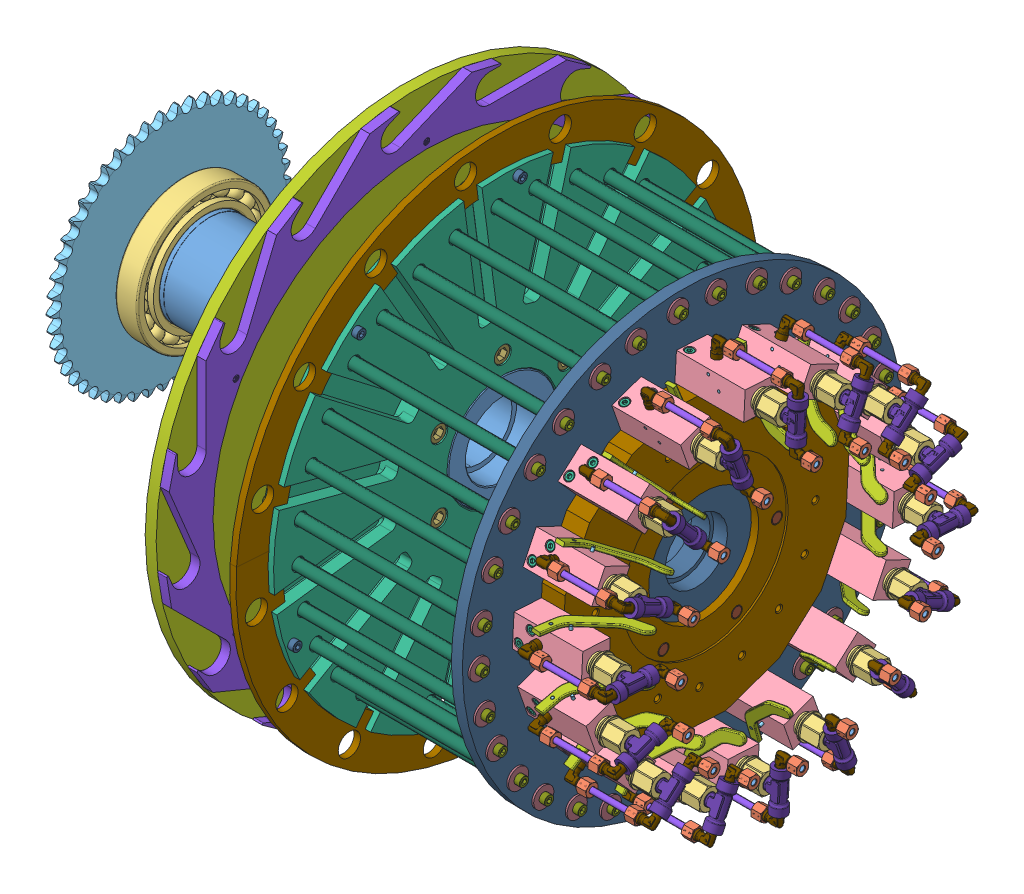
SolidWorks assembly assieme parte rotante, configuration Default. Lengths in mm.
Overall size (749.63 778.63 778.63).
555 component instances, 28 part files, 76 mates.
Components (placement in the parent):
- albero rotazione piatti-1: albero rotazione piatti [Default] at (60.413 18.3637 415) size (415 200 200)
- c-type retaining ring_external_ks-1: c-type retaining ring_external_ks [KS 1336 E - 100] at (-146.4567 18.3637 415) x (0 0 -1) z (1 0 0) size (107.55 112.98 3)
- SKF - 6020 - 20,DE,NC,20_68-1: SKF - 6020 - 20,DE,NC,20_68 [SKF - 6020 - 20,DE,NC,20_68] at (-131.4567 18.3637 415) x (1 0 0) z (0 -0.434476 -0.900684) size (24 150 150)
- calettatore d95-1: calettatore d95 [Default] at (-173.8867 18.3637 415) size (39.5 135 135)
- Chain wheel ISO - 50Z 10A-1-1: Chain wheel ISO - 50Z 10A-1 [Chain wheel ISO - 50Z 10A-1 --50SB120H25L95.0N] at (-164.8867 18.3637 415) size (29.89 262.06 262.51)
- Disco supporto montaggio e Colonne-1: Disco supporto montaggio e Colonne [Default] at (204.0433 18.3637 415) x (0 -0.866025 -0.5) z (1 0 0) size (499.6 499.6 29)
- SKF - 6020 - 20,DE,NC,20_68-2: SKF - 6020 - 20,DE,NC,20_68 [SKF - 6020 - 20,DE,NC,20_68] at (62.0433 18.3637 415) x (1 0 0) z (0 -0.432628 -0.901573) size (24 150 150)
- piatto rotante porta tappi-1: piatto rotante porta tappi [Default] at (99.0433 18.3637 415) x (0 0 -1) z (1 0 0) size (570 570 20.57)
- disco trasportatore tappi 31-1: disco trasportatore tappi 31 [Default] at (111.0433 18.3637 415) x (0 0.5 -0.866025) z (1 0 0) size (570 570 10.42)
- Distributore Rotante-1: Distributore Rotante [Default] at (425.0433 18.3637 415) x (0 -0.055301 -0.99847) z (1 0 0) size (310 310 25.54)
- disco trascinato porta distributore vuoto-1: disco trascinato porta distributore vuoto [Default] at (400.0433 18.3637 415) x (0 0.055301 0.99847) z (-1 0 0) size (480 480 50)
- m12 35mm-1: m12 35mm [ISO 4762 M12 x 35 - 35N] at (376.0433 -53.0243 378.8925) x (1 0 0) z (0 -0.5 0.866025) size (47 18 18)
- m12 90mm-3: m12 90mm [ISO 4762 M12 x 90 - 90N] at (203.0433 -21.6363 345.718) x (-1 0 0) z (0 -0.5 0.866025) size (102 18 18)
- plain washer xlarge grade c_iso-1: plain washer xlarge grade c_iso [Washer ISO 7094 - 6] at (99.0433 -101.6363 207.1539) x (1 0 0) z (0 -1 0) size (2 22 22)
- M6 20mm-1: M6 20mm [ISO 4762 M6 x 20 - 20N] at (91.0433 -101.6363 207.1539) x (1 0 0) z (0 0.5 0.866025) size (26 10 10)
- m12 35mm-2: m12 35mm [ISO 4762 M12 x 35 - 35N] at (376.0433 13.9397 335.1224) x (1 0 0) z (0 -1 0) size (47 18 18)
- m12 35mm-3: m12 35mm [ISO 4762 M12 x 35 - 35N] at (376.0433 85.3277 371.2299) x (1 0 0) z (0 -0.5 -0.866025) size (47 18 18)
- m12 35mm-4: m12 35mm [ISO 4762 M12 x 35 - 35N] at (376.0433 89.7517 451.1075) x (1 0 0) z (0 0.5 -0.866025) size (47 18 18)
- m12 35mm-5: m12 35mm [ISO 4762 M12 x 35 - 35N] at (376.0433 22.7877 494.8776) x (1 0 0) z (0 1 0) size (47 18 18)
- m12 35mm-6: m12 35mm [ISO 4762 M12 x 35 - 35N] at (376.0433 -48.6003 458.7701) x (1 0 0) z (0 0.5 0.866025) size (47 18 18)
- plain washer xlarge grade c_iso-2: plain washer xlarge grade c_iso [Washer ISO 7094 - 6] at (99.0433 138.3637 207.1539) x (1 0 0) z (0 -0.5 -0.866025) size (2 22 22)
- plain washer xlarge grade c_iso-3: plain washer xlarge grade c_iso [Washer ISO 7094 - 6] at (99.0433 258.3637 415) x (1 0 0) z (0 0.5 -0.866025) size (2 22 22)
- plain washer xlarge grade c_iso-4: plain washer xlarge grade c_iso [Washer ISO 7094 - 6] at (99.0433 138.3637 622.8461) x (1 0 0) z (0 1 0) size (2 22 22)
- plain washer xlarge grade c_iso-5: plain washer xlarge grade c_iso [Washer ISO 7094 - 6] at (99.0433 -101.6363 622.8461) x (1 0 0) z (0 0.5 0.866025) size (2 22 22)
- plain washer xlarge grade c_iso-6: plain washer xlarge grade c_iso [Washer ISO 7094 - 6] at (99.0433 -221.6363 415) x (1 0 0) z (0 -0.5 0.866025) size (2 22 22)
- M6 20mm-2: M6 20mm [ISO 4762 M6 x 20 - 20N] at (91.0433 138.3637 207.1539) x (1 0 0) z (0 -0.5 0.866025) size (26 10 10)
- M6 20mm-3: M6 20mm [ISO 4762 M6 x 20 - 20N] at (91.0433 258.3637 415) x (1 0 0) z (0 -1 0) size (26 10 10)
- M6 20mm-4: M6 20mm [ISO 4762 M6 x 20 - 20N] at (91.0433 138.3637 622.8461) x (1 0 0) z (0 -0.5 -0.866025) size (26 10 10)
- M6 20mm-5: M6 20mm [ISO 4762 M6 x 20 - 20N] at (91.0433 -101.6363 622.8461) x (1 0 0) z (0 0.5 -0.866025) size (26 10 10)
- M6 20mm-6: M6 20mm [ISO 4762 M6 x 20 - 20N] at (91.0433 -221.6363 415) x (1 0 0) z (0 1 0) size (26 10 10)
- m12 90mm-4: m12 90mm [ISO 4762 M12 x 90 - 90N] at (203.0433 58.3637 345.718) x (-1 0 0) z (0 -1 0) size (102 18 18)
- m12 90mm-5: m12 90mm [ISO 4762 M12 x 90 - 90N] at (203.0433 98.3637 415) x (-1 0 0) z (0 -0.5 -0.866025) size (102 18 18)
- m12 90mm-6: m12 90mm [ISO 4762 M12 x 90 - 90N] at (203.0433 58.3637 484.282) x (-1 0 0) z (0 0.5 -0.866025) size (102 18 18)
- m12 90mm-7: m12 90mm [ISO 4762 M12 x 90 - 90N] at (203.0433 -21.6363 484.282) x (-1 0 0) z (0 1 0) size (102 18 18)
- m12 90mm-8: m12 90mm [ISO 4762 M12 x 90 - 90N] at (203.0433 -61.6363 415) x (-1 0 0) z (0 0.5 0.866025) size (102 18 18)
- asta scorrimento carello-1: asta scorrimento carello [Default] at (287.5433 70.1437 197.9013) x (0 0 -1) z (1 0 0) size (12 12 225)
- plain washer xlarge grade c_iso-7: plain washer xlarge grade c_iso [Washer ISO 7094 - 6] at (175.0433 70.1437 197.9013) x (1 0 0) z (0 -1 0) size (2 22 22)
- M6 16mm-1: M6 16mm [ISO 4762 M6 x 16 - 16N] at (167.0433 70.1437 197.9013) size (22 10 10)
- M6 16mm-2: M6 16mm [ISO 4762 M6 x 16 - 16N] at (408.0433 70.1437 197.9013) x (-1 0 0) z (0 0 -1) size (22 10 10)
- plain washer xlarge grade c_iso-26: plain washer xlarge grade c_iso [Washer ISO 7094 - 6] at (400.0433 70.1437 197.9013) x (-1 0 0) z (0 1 0) size (2 22 22)
- plain washer xlarge grade c_iso-42: plain washer xlarge grade c_iso [Washer ISO 7094 - 6] at (175.0433 24.5373 191.8971) x (1 0 0) z (0 -0.965926 -0.258819) size (2 22 22)
- M6 16mm-3: M6 16mm [ISO 4762 M6 x 16 - 16N] at (167.0433 24.5373 191.8971) x (1 0 0) z (0 0.258819 -0.965926) size (22 10 10)
- asta scorrimento carello-2: asta scorrimento carello [Default] at (287.5433 24.5373 191.8971) x (0 0.258819 -0.965926) z (-1 0 0) size (12 12 225)
- plain washer xlarge grade c_iso-58: plain washer xlarge grade c_iso [Washer ISO 7094 - 6] at (400.0433 24.5373 191.8971) x (-1 0 0) z (0 0.965926 0.258819) size (2 22 22)
- M6 16mm-4: M6 16mm [ISO 4762 M6 x 16 - 16N] at (408.0433 24.5373 191.8971) x (-1 0 0) z (0 -0.258819 0.965926) size (22 10 10)
- AssiemeValvola-1: AssiemeValvola [Default] at (515.3257 74.6348 254.5832) x (0 -0.331007 0.943628) z (0 0.943628 0.331007) size (90.26 138.63 38)
  - RaccordoT-1: RaccordoT [Default] at origin size (43 29.75 16.5)
  - Raccordo a L-1: Raccordo a L [Default] at (-30 0 0) x (0 -1 0) z (0 0 -1) size (28.34 25.51 14.01)
    - 1809_06_10_01-1: 1809_06_10_01 [Default] at origin size (22.49 23 10)
    - 1809_06_10_02-1: 1809_06_10_02 [Default] at origin size (6.5 8.5 8.5)
    - 1809_06_10_03-1: 1809_06_10_03 [Default] at origin size (11.02 15.01 14.01)
  - Raccordo a L-2: Raccordo a L [Default] at (30 0 0) x (0 1 0) z (0 0 -1) size (28.34 25.51 14.01)
    - 1809_06_10_01-1: 1809_06_10_01 [Default] at origin size (22.49 23 10)
    - 1809_06_10_02-1: 1809_06_10_02 [Default] at origin size (6.5 8.5 8.5)
    - 1809_06_10_03-1: 1809_06_10_03 [Default] at origin size (11.02 15.01 14.01)
  - TappoChiusura-1: TappoChiusura [Default] at (0 -32 0) x (0 -1 0) z (0 0 1) size (38.28 26.74 26.74)
  - CorpoValvola-1: CorpoValvola [Default] at (-15 -115.2824 0) size (30 75 34)
  - Raccordo a L-3: Raccordo a L [Default] at (-30 -88.2824 0) x (0 1 0) z (0 0 1) size (28.34 25.51 14.01)
    - 1809_06_10_01-1: 1809_06_10_01 [Default] at origin size (22.49 23 10)
    - 1809_06_10_02-1: 1809_06_10_02 [Default] at origin size (6.5 8.5 8.5)
    - 1809_06_10_03-1: 1809_06_10_03 [Default] at origin size (11.02 15.01 14.01)
  - Spina_3x38-1: Spina_3x38 [Default] at (0 -68.2824 -21) x (-1 0 0) z (0 0 1) size (3 3 38)
  - Spina_3x38-2: Spina_3x38 [Default] at (-10 -80.2824 -21) x (0.996193 0.087174 0) z (0 0 1) size (3 3 38)
  - M5 40mm-3: M5 40mm [ISO 4762 M5 x 40 - 40N] at (-14.6 -108.7824 9) size (45 8.5 8.5)
  - M5 40mm-2: M5 40mm [ISO 4762 M5 x 40 - 40N] at (-14.6 -96.7824 -9) size (45 8.5 8.5)
  - LevaValvola-1: LevaValvola [Default] at (-24.507 -86.571 -17) x (0.996193 0.087174 0) z (0 0 1) size (77.55 60.2 4)
  - Tubo-1: Tubo [Default] at (-30 -15.9665 0) x (1 0 0) z (0 -1 0) size (6 6 56.4)
- M6 16mm-5: M6 16mm [ISO 4762 M6 x 16 - 16N] at (167.0433 -16.8778 194.6116) x (1 0 0) z (0 0.382683 0.92388) size (22 10 10)
- M6 16mm-6: M6 16mm [ISO 4762 M6 x 16 - 16N] at (167.0433 -98.5342 224.874) x (1 0 0) z (0 0.707107 0.707107) size (22 10 10)
- M6 16mm-7: M6 16mm [ISO 4762 M6 x 16 - 16N] at (167.0433 -162.3939 284.0814) x (1 0 0) z (0 0.92388 0.382683) size (22 10 10)
- M6 16mm-8: M6 16mm [ISO 4762 M6 x 16 - 16N] at (167.0433 -198.735 363.22) x (1 0 0) z (0 1 0) size (22 10 10)
- M6 16mm-9: M6 16mm [ISO 4762 M6 x 16 - 16N] at (167.0433 -202.0247 450.2415) x (1 0 0) z (0 0.92388 -0.382683) size (22 10 10)
- M6 16mm-10: M6 16mm [ISO 4762 M6 x 16 - 16N] at (167.0433 -171.7623 531.8979) x (1 0 0) z (0 0.707107 -0.707107) size (22 10 10)
- M6 16mm-11: M6 16mm [ISO 4762 M6 x 16 - 16N] at (167.0433 -112.5549 595.7576) x (1 0 0) z (0 0.382683 -0.92388) size (22 10 10)
- M6 16mm-12: M6 16mm [ISO 4762 M6 x 16 - 16N] at (167.0433 -33.4163 632.0987) x (1 0 0) z (0 0 -1) size (22 10 10)
- M6 16mm-13: M6 16mm [ISO 4762 M6 x 16 - 16N] at (167.0433 53.6052 635.3884) x (1 0 0) z (0 -0.382683 -0.92388) size (22 10 10)
- M6 16mm-14: M6 16mm [ISO 4762 M6 x 16 - 16N] at (167.0433 135.2616 605.126) x (1 0 0) z (0 -0.707107 -0.707107) size (22 10 10)
- M6 16mm-15: M6 16mm [ISO 4762 M6 x 16 - 16N] at (167.0433 199.1213 545.9186) x (1 0 0) z (0 -0.92388 -0.382683) size (22 10 10)
- M6 16mm-16: M6 16mm [ISO 4762 M6 x 16 - 16N] at (167.0433 235.4624 466.78) x (1 0 0) z (0 -1 0) size (22 10 10)
- M6 16mm-17: M6 16mm [ISO 4762 M6 x 16 - 16N] at (167.0433 238.7521 379.7585) x (1 0 0) z (0 -0.92388 0.382683) size (22 10 10)
- M6 16mm-18: M6 16mm [ISO 4762 M6 x 16 - 16N] at (167.0433 208.4897 298.1021) x (1 0 0) z (0 -0.707107 0.707107) size (22 10 10)
- M6 16mm-19: M6 16mm [ISO 4762 M6 x 16 - 16N] at (167.0433 149.2823 234.2424) x (1 0 0) z (0 -0.382683 0.92388) size (22 10 10)
- plain washer xlarge grade c_iso-11: plain washer xlarge grade c_iso [Washer ISO 7094 - 6] at (175.0433 -16.8778 194.6116) x (1 0 0) z (0 -0.92388 0.382683) size (2 22 22)
- plain washer xlarge grade c_iso-12: plain washer xlarge grade c_iso [Washer ISO 7094 - 6] at (175.0433 -98.5342 224.874) x (1 0 0) z (0 -0.707107 0.707107) size (2 22 22)
- plain washer xlarge grade c_iso-13: plain washer xlarge grade c_iso [Washer ISO 7094 - 6] at (175.0433 -162.3939 284.0814) x (1 0 0) z (0 -0.382683 0.92388) size (2 22 22)
- plain washer xlarge grade c_iso-14: plain washer xlarge grade c_iso [Washer ISO 7094 - 6] at (175.0433 -198.735 363.22) size (2 22 22)
- plain washer xlarge grade c_iso-15: plain washer xlarge grade c_iso [Washer ISO 7094 - 6] at (175.0433 -202.0247 450.2415) x (1 0 0) z (0 0.382683 0.92388) size (2 22 22)
- plain washer xlarge grade c_iso-16: plain washer xlarge grade c_iso [Washer ISO 7094 - 6] at (175.0433 -171.7623 531.8979) x (1 0 0) z (0 0.707107 0.707107) size (2 22 22)
- plain washer xlarge grade c_iso-17: plain washer xlarge grade c_iso [Washer ISO 7094 - 6] at (175.0433 -112.5549 595.7576) x (1 0 0) z (0 0.92388 0.382683) size (2 22 22)
- plain washer xlarge grade c_iso-18: plain washer xlarge grade c_iso [Washer ISO 7094 - 6] at (175.0433 -33.4163 632.0987) x (1 0 0) z (0 1 0) size (2 22 22)
- plain washer xlarge grade c_iso-19: plain washer xlarge grade c_iso [Washer ISO 7094 - 6] at (175.0433 53.6052 635.3884) x (1 0 0) z (0 0.92388 -0.382683) size (2 22 22)
- plain washer xlarge grade c_iso-20: plain washer xlarge grade c_iso [Washer ISO 7094 - 6] at (175.0433 135.2616 605.126) x (1 0 0) z (0 0.707107 -0.707107) size (2 22 22)
- plain washer xlarge grade c_iso-21: plain washer xlarge grade c_iso [Washer ISO 7094 - 6] at (175.0433 199.1213 545.9186) x (1 0 0) z (0 0.382683 -0.92388) size (2 22 22)
- plain washer xlarge grade c_iso-22: plain washer xlarge grade c_iso [Washer ISO 7094 - 6] at (175.0433 235.4624 466.78) x (1 0 0) z (0 0 -1) size (2 22 22)
- plain washer xlarge grade c_iso-23: plain washer xlarge grade c_iso [Washer ISO 7094 - 6] at (175.0433 238.7521 379.7585) x (1 0 0) z (0 -0.382683 -0.92388) size (2 22 22)
- plain washer xlarge grade c_iso-24: plain washer xlarge grade c_iso [Washer ISO 7094 - 6] at (175.0433 208.4897 298.1021) x (1 0 0) z (0 -0.707107 -0.707107) size (2 22 22)
- plain washer xlarge grade c_iso-25: plain washer xlarge grade c_iso [Washer ISO 7094 - 6] at (175.0433 149.2823 234.2424) x (1 0 0) z (0 -0.92388 -0.382683) size (2 22 22)
- asta scorrimento carello-3: asta scorrimento carello [Default] at (287.5433 -16.8778 194.6116) x (0 -0.382683 -0.92388) z (1 0 0) size (12 12 225)
- asta scorrimento carello-4: asta scorrimento carello [Default] at (287.5433 -98.5342 224.874) x (0 -0.707107 -0.707107) z (1 0 0) size (12 12 225)
- asta scorrimento carello-5: asta scorrimento carello [Default] at (287.5433 -162.3939 284.0814) x (0 -0.92388 -0.382683) z (1 0 0) size (12 12 225)
- asta scorrimento carello-6: asta scorrimento carello [Default] at (287.5433 -198.735 363.22) x (0 -1 0) z (1 0 0) size (12 12 225)
- asta scorrimento carello-7: asta scorrimento carello [Default] at (287.5433 -202.0247 450.2415) x (0 -0.92388 0.382683) z (1 0 0) size (12 12 225)
- asta scorrimento carello-8: asta scorrimento carello [Default] at (287.5433 -171.7623 531.8979) x (0 -0.707107 0.707107) z (1 0 0) size (12 12 225)
- asta scorrimento carello-9: asta scorrimento carello [Default] at (287.5433 -112.5549 595.7576) x (0 -0.382683 0.92388) z (1 0 0) size (12 12 225)
- asta scorrimento carello-10: asta scorrimento carello [Default] at (287.5433 -33.4163 632.0987) x (0 0 1) z (1 0 0) size (12 12 225)
- asta scorrimento carello-11: asta scorrimento carello [Default] at (287.5433 53.6052 635.3884) x (0 0.382683 0.92388) z (1 0 0) size (12 12 225)
- asta scorrimento carello-12: asta scorrimento carello [Default] at (287.5433 135.2616 605.126) x (0 0.707107 0.707107) z (1 0 0) size (12 12 225)
- asta scorrimento carello-13: asta scorrimento carello [Default] at (287.5433 199.1213 545.9186) x (0 0.92388 0.382683) z (1 0 0) size (12 12 225)
- asta scorrimento carello-14: asta scorrimento carello [Default] at (287.5433 235.4624 466.78) x (0 1 0) z (1 0 0) size (12 12 225)
- asta scorrimento carello-15: asta scorrimento carello [Default] at (287.5433 238.7521 379.7585) x (0 0.92388 -0.382683) z (1 0 0) size (12 12 225)
- asta scorrimento carello-16: asta scorrimento carello [Default] at (287.5433 208.4897 298.1021) x (0 0.707107 -0.707107) z (1 0 0) size (12 12 225)
- asta scorrimento carello-17: asta scorrimento carello [Default] at (287.5433 149.2823 234.2424) x (0 0.382683 -0.92388) z (1 0 0) size (12 12 225)
- M6 16mm-20: M6 16mm [ISO 4762 M6 x 16 - 16N] at (408.0433 -16.8778 194.6116) x (-1 0 0) z (0 -0.382683 -0.92388) size (22 10 10)
- M6 16mm-21: M6 16mm [ISO 4762 M6 x 16 - 16N] at (408.0433 -98.5342 224.874) x (-1 0 0) z (0 -0.707107 -0.707107) size (22 10 10)
- M6 16mm-22: M6 16mm [ISO 4762 M6 x 16 - 16N] at (408.0433 -162.3939 284.0814) x (-1 0 0) z (0 -0.92388 -0.382683) size (22 10 10)
- M6 16mm-23: M6 16mm [ISO 4762 M6 x 16 - 16N] at (408.0433 -198.735 363.22) x (-1 0 0) z (0 -1 0) size (22 10 10)
- M6 16mm-24: M6 16mm [ISO 4762 M6 x 16 - 16N] at (408.0433 -202.0247 450.2415) x (-1 0 0) z (0 -0.92388 0.382683) size (22 10 10)
- M6 16mm-25: M6 16mm [ISO 4762 M6 x 16 - 16N] at (408.0433 -171.7623 531.8979) x (-1 0 0) z (0 -0.707107 0.707107) size (22 10 10)
- M6 16mm-26: M6 16mm [ISO 4762 M6 x 16 - 16N] at (408.0433 -112.5549 595.7576) x (-1 0 0) z (0 -0.382683 0.92388) size (22 10 10)
- M6 16mm-27: M6 16mm [ISO 4762 M6 x 16 - 16N] at (408.0433 -33.4163 632.0987) x (-1 0 0) z (0 0 1) size (22 10 10)
- M6 16mm-28: M6 16mm [ISO 4762 M6 x 16 - 16N] at (408.0433 53.6052 635.3884) x (-1 0 0) z (0 0.382683 0.92388) size (22 10 10)
- M6 16mm-29: M6 16mm [ISO 4762 M6 x 16 - 16N] at (408.0433 135.2616 605.126) x (-1 0 0) z (0 0.707107 0.707107) size (22 10 10)
- M6 16mm-30: M6 16mm [ISO 4762 M6 x 16 - 16N] at (408.0433 199.1213 545.9186) x (-1 0 0) z (0 0.92388 0.382683) size (22 10 10)
- M6 16mm-31: M6 16mm [ISO 4762 M6 x 16 - 16N] at (408.0433 235.4624 466.78) x (-1 0 0) z (0 1 0) size (22 10 10)
- M6 16mm-32: M6 16mm [ISO 4762 M6 x 16 - 16N] at (408.0433 238.7521 379.7585) x (-1 0 0) z (0 0.92388 -0.382683) size (22 10 10)
- M6 16mm-33: M6 16mm [ISO 4762 M6 x 16 - 16N] at (408.0433 208.4897 298.1021) x (-1 0 0) z (0 0.707107 -0.707107) size (22 10 10)
- M6 16mm-34: M6 16mm [ISO 4762 M6 x 16 - 16N] at (408.0433 149.2823 234.2424) x (-1 0 0) z (0 0.382683 -0.92388) size (22 10 10)
- plain washer xlarge grade c_iso-27: plain washer xlarge grade c_iso [Washer ISO 7094 - 6] at (400.0433 -16.8778 194.6116) x (-1 0 0) z (0 0.92388 -0.382683) size (2 22 22)
- plain washer xlarge grade c_iso-28: plain washer xlarge grade c_iso [Washer ISO 7094 - 6] at (400.0433 -98.5342 224.874) x (-1 0 0) z (0 0.707107 -0.707107) size (2 22 22)
- plain washer xlarge grade c_iso-29: plain washer xlarge grade c_iso [Washer ISO 7094 - 6] at (400.0433 -162.3939 284.0814) x (-1 0 0) z (0 0.382683 -0.92388) size (2 22 22)
- plain washer xlarge grade c_iso-30: plain washer xlarge grade c_iso [Washer ISO 7094 - 6] at (400.0433 -198.735 363.22) x (-1 0 0) z (0 0 -1) size (2 22 22)
- plain washer xlarge grade c_iso-31: plain washer xlarge grade c_iso [Washer ISO 7094 - 6] at (400.0433 -202.0247 450.2415) x (-1 0 0) z (0 -0.382683 -0.92388) size (2 22 22)
- plain washer xlarge grade c_iso-32: plain washer xlarge grade c_iso [Washer ISO 7094 - 6] at (400.0433 -171.7623 531.8979) x (-1 0 0) z (0 -0.707107 -0.707107) size (2 22 22)
- plain washer xlarge grade c_iso-33: plain washer xlarge grade c_iso [Washer ISO 7094 - 6] at (400.0433 -112.5549 595.7576) x (-1 0 0) z (0 -0.92388 -0.382683) size (2 22 22)
- plain washer xlarge grade c_iso-34: plain washer xlarge grade c_iso [Washer ISO 7094 - 6] at (400.0433 -33.4163 632.0987) x (-1 0 0) z (0 -1 0) size (2 22 22)
- plain washer xlarge grade c_iso-35: plain washer xlarge grade c_iso [Washer ISO 7094 - 6] at (400.0433 53.6052 635.3884) x (-1 0 0) z (0 -0.92388 0.382683) size (2 22 22)
- plain washer xlarge grade c_iso-36: plain washer xlarge grade c_iso [Washer ISO 7094 - 6] at (400.0433 135.2616 605.126) x (-1 0 0) z (0 -0.707107 0.707107) size (2 22 22)
- plain washer xlarge grade c_iso-37: plain washer xlarge grade c_iso [Washer ISO 7094 - 6] at (400.0433 199.1213 545.9186) x (-1 0 0) z (0 -0.382683 0.92388) size (2 22 22)
- plain washer xlarge grade c_iso-38: plain washer xlarge grade c_iso [Washer ISO 7094 - 6] at (400.0433 235.4624 466.78) x (-1 0 0) z (0 0 1) size (2 22 22)
- plain washer xlarge grade c_iso-39: plain washer xlarge grade c_iso [Washer ISO 7094 - 6] at (400.0433 238.7521 379.7585) x (-1 0 0) z (0 0.382683 0.92388) size (2 22 22)
- plain washer xlarge grade c_iso-40: plain washer xlarge grade c_iso [Washer ISO 7094 - 6] at (400.0433 208.4897 298.1021) x (-1 0 0) z (0 0.707107 0.707107) size (2 22 22)
- plain washer xlarge grade c_iso-41: plain washer xlarge grade c_iso [Washer ISO 7094 - 6] at (400.0433 149.2823 234.2424) x (-1 0 0) z (0 0.92388 0.382683) size (2 22 22)
- plain washer xlarge grade c_iso-43: plain washer xlarge grade c_iso [Washer ISO 7094 - 6] at (175.0433 -61.3104 206.5173) x (1 0 0) z (0 -0.991445 0.130526) size (2 22 22)
- plain washer xlarge grade c_iso-44: plain washer xlarge grade c_iso [Washer ISO 7094 - 6] at (175.0433 -135.0285 252.8771) x (1 0 0) z (0 -0.866025 0.5) size (2 22 22)
- plain washer xlarge grade c_iso-45: plain washer xlarge grade c_iso [Washer ISO 7094 - 6] at (175.0433 -185.3939 323.9186) x (1 0 0) z (0 -0.608761 0.793353) size (2 22 22)
- plain washer xlarge grade c_iso-46: plain washer xlarge grade c_iso [Washer ISO 7094 - 6] at (175.0433 -204.7392 408.8264) x (1 0 0) z (0 -0.258819 0.965926) size (2 22 22)
- plain washer xlarge grade c_iso-47: plain washer xlarge grade c_iso [Washer ISO 7094 - 6] at (175.0433 -190.119 494.6741) x (1 0 0) z (0 0.130526 0.991445) size (2 22 22)
- plain washer xlarge grade c_iso-48: plain washer xlarge grade c_iso [Washer ISO 7094 - 6] at (175.0433 -143.7592 568.3922) x (1 0 0) z (0 0.5 0.866025) size (2 22 22)
- plain washer xlarge grade c_iso-49: plain washer xlarge grade c_iso [Washer ISO 7094 - 6] at (175.0433 -72.7177 618.7576) x (1 0 0) z (0 0.793353 0.608761) size (2 22 22)
- plain washer xlarge grade c_iso-50: plain washer xlarge grade c_iso [Washer ISO 7094 - 6] at (175.0433 12.1901 638.1029) x (1 0 0) z (0 0.965926 0.258819) size (2 22 22)
- plain washer xlarge grade c_iso-51: plain washer xlarge grade c_iso [Washer ISO 7094 - 6] at (175.0433 98.0378 623.4827) x (1 0 0) z (0 0.991445 -0.130526) size (2 22 22)
- plain washer xlarge grade c_iso-52: plain washer xlarge grade c_iso [Washer ISO 7094 - 6] at (175.0433 171.7559 577.1229) x (1 0 0) z (0 0.866025 -0.5) size (2 22 22)
- plain washer xlarge grade c_iso-53: plain washer xlarge grade c_iso [Washer ISO 7094 - 6] at (175.0433 222.1213 506.0814) x (1 0 0) z (0 0.608761 -0.793353) size (2 22 22)
- plain washer xlarge grade c_iso-54: plain washer xlarge grade c_iso [Washer ISO 7094 - 6] at (175.0433 241.4666 421.1736) x (1 0 0) z (0 0.258819 -0.965926) size (2 22 22)
- plain washer xlarge grade c_iso-55: plain washer xlarge grade c_iso [Washer ISO 7094 - 6] at (175.0433 226.8464 335.3259) x (1 0 0) z (0 -0.130526 -0.991445) size (2 22 22)
- plain washer xlarge grade c_iso-56: plain washer xlarge grade c_iso [Washer ISO 7094 - 6] at (175.0433 180.4866 261.6078) x (1 0 0) z (0 -0.5 -0.866025) size (2 22 22)
- plain washer xlarge grade c_iso-57: plain washer xlarge grade c_iso [Washer ISO 7094 - 6] at (175.0433 109.4451 211.2424) x (1 0 0) z (0 -0.793353 -0.608761) size (2 22 22)
- M6 16mm-35: M6 16mm [ISO 4762 M6 x 16 - 16N] at (167.0433 -61.3104 206.5173) x (1 0 0) z (0 -0.130526 -0.991445) size (22 10 10)
- M6 16mm-36: M6 16mm [ISO 4762 M6 x 16 - 16N] at (167.0433 -135.0285 252.8771) x (1 0 0) z (0 -0.5 -0.866025) size (22 10 10)
- M6 16mm-37: M6 16mm [ISO 4762 M6 x 16 - 16N] at (167.0433 -185.3939 323.9186) x (1 0 0) z (0 -0.793353 -0.608761) size (22 10 10)
- M6 16mm-38: M6 16mm [ISO 4762 M6 x 16 - 16N] at (167.0433 -204.7392 408.8264) x (1 0 0) z (0 -0.965926 -0.258819) size (22 10 10)
- M6 16mm-39: M6 16mm [ISO 4762 M6 x 16 - 16N] at (167.0433 -190.119 494.6741) x (1 0 0) z (0 -0.991445 0.130526) size (22 10 10)
- M6 16mm-40: M6 16mm [ISO 4762 M6 x 16 - 16N] at (167.0433 -143.7592 568.3922) x (1 0 0) z (0 -0.866025 0.5) size (22 10 10)
- M6 16mm-41: M6 16mm [ISO 4762 M6 x 16 - 16N] at (167.0433 -72.7177 618.7576) x (1 0 0) z (0 -0.608761 0.793353) size (22 10 10)
- M6 16mm-42: M6 16mm [ISO 4762 M6 x 16 - 16N] at (167.0433 12.1901 638.1029) x (1 0 0) z (0 -0.258819 0.965926) size (22 10 10)
- M6 16mm-43: M6 16mm [ISO 4762 M6 x 16 - 16N] at (167.0433 98.0378 623.4827) x (1 0 0) z (0 0.130526 0.991445) size (22 10 10)
- M6 16mm-44: M6 16mm [ISO 4762 M6 x 16 - 16N] at (167.0433 171.7559 577.1229) x (1 0 0) z (0 0.5 0.866025) size (22 10 10)
- M6 16mm-45: M6 16mm [ISO 4762 M6 x 16 - 16N] at (167.0433 222.1213 506.0814) x (1 0 0) z (0 0.793353 0.608761) size (22 10 10)
- M6 16mm-46: M6 16mm [ISO 4762 M6 x 16 - 16N] at (167.0433 241.4666 421.1736) x (1 0 0) z (0 0.965926 0.258819) size (22 10 10)
- M6 16mm-47: M6 16mm [ISO 4762 M6 x 16 - 16N] at (167.0433 226.8464 335.3259) x (1 0 0) z (0 0.991445 -0.130526) size (22 10 10)
- M6 16mm-48: M6 16mm [ISO 4762 M6 x 16 - 16N] at (167.0433 180.4866 261.6078) x (1 0 0) z (0 0.866025 -0.5) size (22 10 10)
- M6 16mm-49: M6 16mm [ISO 4762 M6 x 16 - 16N] at (167.0433 109.4451 211.2424) x (1 0 0) z (0 0.608761 -0.793353) size (22 10 10)
- asta scorrimento carello-18: asta scorrimento carello [Default] at (287.5433 -61.3104 206.5173) x (0 -0.130526 -0.991445) z (-1 0 0) size (12 12 225)
- asta scorrimento carello-19: asta scorrimento carello [Default] at (287.5433 -135.0285 252.8771) x (0 -0.5 -0.866025) z (-1 0 0) size (12 12 225)
- asta scorrimento carello-20: asta scorrimento carello [Default] at (287.5433 -185.3939 323.9186) x (0 -0.793353 -0.608761) z (-1 0 0) size (12 12 225)
- asta scorrimento carello-21: asta scorrimento carello [Default] at (287.5433 -204.7392 408.8264) x (0 -0.965926 -0.258819) z (-1 0 0) size (12 12 225)
- asta scorrimento carello-22: asta scorrimento carello [Default] at (287.5433 -190.119 494.6741) x (0 -0.991445 0.130526) z (-1 0 0) size (12 12 225)
- asta scorrimento carello-23: asta scorrimento carello [Default] at (287.5433 -143.7592 568.3922) x (0 -0.866025 0.5) z (-1 0 0) size (12 12 225)
- asta scorrimento carello-24: asta scorrimento carello [Default] at (287.5433 -72.7177 618.7576) x (0 -0.608761 0.793353) z (-1 0 0) size (12 12 225)
- asta scorrimento carello-25: asta scorrimento carello [Default] at (287.5433 12.1901 638.1029) x (0 -0.258819 0.965926) z (-1 0 0) size (12 12 225)
- asta scorrimento carello-26: asta scorrimento carello [Default] at (287.5433 98.0378 623.4827) x (0 0.130526 0.991445) z (-1 0 0) size (12 12 225)
- asta scorrimento carello-27: asta scorrimento carello [Default] at (287.5433 171.7559 577.1229) x (0 0.5 0.866025) z (-1 0 0) size (12 12 225)
- asta scorrimento carello-28: asta scorrimento carello [Default] at (287.5433 222.1213 506.0814) x (0 0.793353 0.608761) z (-1 0 0) size (12 12 225)
- asta scorrimento carello-29: asta scorrimento carello [Default] at (287.5433 241.4666 421.1736) x (0 0.965926 0.258819) z (-1 0 0) size (12 12 225)
- asta scorrimento carello-30: asta scorrimento carello [Default] at (287.5433 226.8464 335.3259) x (0 0.991445 -0.130526) z (-1 0 0) size (12 12 225)
- asta scorrimento carello-31: asta scorrimento carello [Default] at (287.5433 180.4866 261.6078) x (0 0.866025 -0.5) z (-1 0 0) size (12 12 225)
- asta scorrimento carello-32: asta scorrimento carello [Default] at (287.5433 109.4451 211.2424) x (0 0.608761 -0.793353) z (-1 0 0) size (12 12 225)
- plain washer xlarge grade c_iso-59: plain washer xlarge grade c_iso [Washer ISO 7094 - 6] at (400.0433 -61.3104 206.5173) x (-1 0 0) z (0 0.991445 -0.130526) size (2 22 22)
- plain washer xlarge grade c_iso-60: plain washer xlarge grade c_iso [Washer ISO 7094 - 6] at (400.0433 -135.0285 252.8771) x (-1 0 0) z (0 0.866025 -0.5) size (2 22 22)
- plain washer xlarge grade c_iso-61: plain washer xlarge grade c_iso [Washer ISO 7094 - 6] at (400.0433 -185.3939 323.9186) x (-1 0 0) z (0 0.608761 -0.793353) size (2 22 22)
- plain washer xlarge grade c_iso-62: plain washer xlarge grade c_iso [Washer ISO 7094 - 6] at (400.0433 -204.7392 408.8264) x (-1 0 0) z (0 0.258819 -0.965926) size (2 22 22)
- plain washer xlarge grade c_iso-63: plain washer xlarge grade c_iso [Washer ISO 7094 - 6] at (400.0433 -190.119 494.6741) x (-1 0 0) z (0 -0.130526 -0.991445) size (2 22 22)
- plain washer xlarge grade c_iso-64: plain washer xlarge grade c_iso [Washer ISO 7094 - 6] at (400.0433 -143.7592 568.3922) x (-1 0 0) z (0 -0.5 -0.866025) size (2 22 22)
- plain washer xlarge grade c_iso-65: plain washer xlarge grade c_iso [Washer ISO 7094 - 6] at (400.0433 -72.7177 618.7576) x (-1 0 0) z (0 -0.793353 -0.608761) size (2 22 22)
- plain washer xlarge grade c_iso-66: plain washer xlarge grade c_iso [Washer ISO 7094 - 6] at (400.0433 12.1901 638.1029) x (-1 0 0) z (0 -0.965926 -0.258819) size (2 22 22)
- plain washer xlarge grade c_iso-67: plain washer xlarge grade c_iso [Washer ISO 7094 - 6] at (400.0433 98.0378 623.4827) x (-1 0 0) z (0 -0.991445 0.130526) size (2 22 22)
- plain washer xlarge grade c_iso-68: plain washer xlarge grade c_iso [Washer ISO 7094 - 6] at (400.0433 171.7559 577.1229) x (-1 0 0) z (0 -0.866025 0.5) size (2 22 22)
- plain washer xlarge grade c_iso-69: plain washer xlarge grade c_iso [Washer ISO 7094 - 6] at (400.0433 222.1213 506.0814) x (-1 0 0) z (0 -0.608761 0.793353) size (2 22 22)
- plain washer xlarge grade c_iso-70: plain washer xlarge grade c_iso [Washer ISO 7094 - 6] at (400.0433 241.4666 421.1736) x (-1 0 0) z (0 -0.258819 0.965926) size (2 22 22)
- plain washer xlarge grade c_iso-71: plain washer xlarge grade c_iso [Washer ISO 7094 - 6] at (400.0433 226.8464 335.3259) x (-1 0 0) z (0 0.130526 0.991445) size (2 22 22)
- plain washer xlarge grade c_iso-72: plain washer xlarge grade c_iso [Washer ISO 7094 - 6] at (400.0433 180.4866 261.6078) x (-1 0 0) z (0 0.5 0.866025) size (2 22 22)
- plain washer xlarge grade c_iso-73: plain washer xlarge grade c_iso [Washer ISO 7094 - 6] at (400.0433 109.4451 211.2424) x (-1 0 0) z (0 0.793353 0.608761) size (2 22 22)
- M6 16mm-50: M6 16mm [ISO 4762 M6 x 16 - 16N] at (408.0433 -61.3104 206.5173) x (-1 0 0) z (0 0.130526 0.991445) size (22 10 10)
- M6 16mm-51: M6 16mm [ISO 4762 M6 x 16 - 16N] at (408.0433 -135.0285 252.8771) x (-1 0 0) z (0 0.5 0.866025) size (22 10 10)
- M6 16mm-52: M6 16mm [ISO 4762 M6 x 16 - 16N] at (408.0433 -185.3939 323.9186) x (-1 0 0) z (0 0.793353 0.608761) size (22 10 10)
- M6 16mm-53: M6 16mm [ISO 4762 M6 x 16 - 16N] at (408.0433 -204.7392 408.8264) x (-1 0 0) z (0 0.965926 0.258819) size (22 10 10)
- M6 16mm-54: M6 16mm [ISO 4762 M6 x 16 - 16N] at (408.0433 -190.119 494.6741) x (-1 0 0) z (0 0.991445 -0.130526) size (22 10 10)
- M6 16mm-55: M6 16mm [ISO 4762 M6 x 16 - 16N] at (408.0433 -143.7592 568.3922) x (-1 0 0) z (0 0.866025 -0.5) size (22 10 10)
- M6 16mm-56: M6 16mm [ISO 4762 M6 x 16 - 16N] at (408.0433 -72.7177 618.7576) x (-1 0 0) z (0 0.608761 -0.793353) size (22 10 10)
- M6 16mm-57: M6 16mm [ISO 4762 M6 x 16 - 16N] at (408.0433 12.1901 638.1029) x (-1 0 0) z (0 0.258819 -0.965926) size (22 10 10)
- M6 16mm-58: M6 16mm [ISO 4762 M6 x 16 - 16N] at (408.0433 98.0378 623.4827) x (-1 0 0) z (0 -0.130526 -0.991445) size (22 10 10)
- M6 16mm-59: M6 16mm [ISO 4762 M6 x 16 - 16N] at (408.0433 171.7559 577.1229) x (-1 0 0) z (0 -0.5 -0.866025) size (22 10 10)
- M6 16mm-60: M6 16mm [ISO 4762 M6 x 16 - 16N] at (408.0433 222.1213 506.0814) x (-1 0 0) z (0 -0.793353 -0.608761) size (22 10 10)
- M6 16mm-61: M6 16mm [ISO 4762 M6 x 16 - 16N] at (408.0433 241.4666 421.1736) x (-1 0 0) z (0 -0.965926 -0.258819) size (22 10 10)
- M6 16mm-62: M6 16mm [ISO 4762 M6 x 16 - 16N] at (408.0433 226.8464 335.3259) x (-1 0 0) z (0 -0.991445 0.130526) size (22 10 10)
- M6 16mm-63: M6 16mm [ISO 4762 M6 x 16 - 16N] at (408.0433 180.4866 261.6078) x (-1 0 0) z (0 -0.866025 0.5) size (22 10 10)
- M6 16mm-64: M6 16mm [ISO 4762 M6 x 16 - 16N] at (408.0433 109.4451 211.2424) x (-1 0 0) z (0 -0.608761 0.793353) size (22 10 10)
- AssiemeValvola-2: AssiemeValvola [Default] at (515.3257 8.9626 245.2601) x (0 0.055301 0.99847) z (0 0.99847 -0.055301) size (90.26 138.63 38)
  - RaccordoT-1: RaccordoT [Default] at origin size (43 29.75 16.5)
  - Raccordo a L-1: Raccordo a L [Default] at (-30 0 0) x (0 -1 0) z (0 0 -1) size (28.34 25.51 14.01)
    - 1809_06_10_01-1: 1809_06_10_01 [Default] at origin size (22.49 23 10)
    - 1809_06_10_02-1: 1809_06_10_02 [Default] at origin size (6.5 8.5 8.5)
    - 1809_06_10_03-1: 1809_06_10_03 [Default] at origin size (11.02 15.01 14.01)
  - Raccordo a L-2: Raccordo a L [Default] at (30 0 0) x (0 1 0) z (0 0 -1) size (28.34 25.51 14.01)
    - 1809_06_10_01-1: 1809_06_10_01 [Default] at origin size (22.49 23 10)
    - 1809_06_10_02-1: 1809_06_10_02 [Default] at origin size (6.5 8.5 8.5)
    - 1809_06_10_03-1: 1809_06_10_03 [Default] at origin size (11.02 15.01 14.01)
  - TappoChiusura-1: TappoChiusura [Default] at (0 -32 0) x (0 -1 0) z (0 0 1) size (38.28 26.74 26.74)
  - CorpoValvola-1: CorpoValvola [Default] at (-15 -115.2824 0) size (30 75 34)
  - Raccordo a L-3: Raccordo a L [Default] at (-30 -88.2824 0) x (0 1 0) z (0 0 1) size (28.34 25.51 14.01)
    - 1809_06_10_01-1: 1809_06_10_01 [Default] at origin size (22.49 23 10)
    - 1809_06_10_02-1: 1809_06_10_02 [Default] at origin size (6.5 8.5 8.5)
    - 1809_06_10_03-1: 1809_06_10_03 [Default] at origin size (11.02 15.01 14.01)
  - Spina_3x38-1: Spina_3x38 [Default] at (0 -68.2824 -21) x (-1 0 0) z (0 0 1) size (3 3 38)
  - Spina_3x38-2: Spina_3x38 [Default] at (-10 -80.2824 -21) x (0.996193 0.087174 0) z (0 0 1) size (3 3 38)
  - M5 40mm-3: M5 40mm [ISO 4762 M5 x 40 - 40N] at (-14.6 -108.7824 9) size (45 8.5 8.5)
  - M5 40mm-2: M5 40mm [ISO 4762 M5 x 40 - 40N] at (-14.6 -96.7824 -9) size (45 8.5 8.5)
  - LevaValvola-1: LevaValvola [Default] at (-24.507 -86.571 -17) x (0.996193 0.087174 0) z (0 0 1) size (77.55 60.2 4)
  - Tubo-1: Tubo [Default] at (-30 -15.9665 0) x (1 0 0) z (0 -1 0) size (6 6 56.4)
- AssiemeValvola-3: AssiemeValvola [Default] at (515.3257 -55.2784 261.7785) x (0 0.433189 0.901303) z (0 0.901303 -0.433189) size (90.26 138.63 38)
  - RaccordoT-1: RaccordoT [Default] at origin size (43 29.75 16.5)
  - Raccordo a L-1: Raccordo a L [Default] at (-30 0 0) x (0 -1 0) z (0 0 -1) size (28.34 25.51 14.01)
    - 1809_06_10_01-1: 1809_06_10_01 [Default] at origin size (22.49 23 10)
    - 1809_06_10_02-1: 1809_06_10_02 [Default] at origin size (6.5 8.5 8.5)
    - 1809_06_10_03-1: 1809_06_10_03 [Default] at origin size (11.02 15.01 14.01)
  - Raccordo a L-2: Raccordo a L [Default] at (30 0 0) x (0 1 0) z (0 0 -1) size (28.34 25.51 14.01)
    - 1809_06_10_01-1: 1809_06_10_01 [Default] at origin size (22.49 23 10)
    - 1809_06_10_02-1: 1809_06_10_02 [Default] at origin size (6.5 8.5 8.5)
    - 1809_06_10_03-1: 1809_06_10_03 [Default] at origin size (11.02 15.01 14.01)
  - TappoChiusura-1: TappoChiusura [Default] at (0 -32 0) x (0 -1 0) z (0 0 1) size (38.28 26.74 26.74)
  - CorpoValvola-1: CorpoValvola [Default] at (-15 -115.2824 0) size (30 75 34)
  - Raccordo a L-3: Raccordo a L [Default] at (-30 -88.2824 0) x (0 1 0) z (0 0 1) size (28.34 25.51 14.01)
    - 1809_06_10_01-1: 1809_06_10_01 [Default] at origin size (22.49 23 10)
    - 1809_06_10_02-1: 1809_06_10_02 [Default] at origin size (6.5 8.5 8.5)
    - 1809_06_10_03-1: 1809_06_10_03 [Default] at origin size (11.02 15.01 14.01)
  - Spina_3x38-1: Spina_3x38 [Default] at (0 -68.2824 -21) x (-1 0 0) z (0 0 1) size (3 3 38)
  - Spina_3x38-2: Spina_3x38 [Default] at (-10 -80.2824 -21) x (0.996193 0.087174 0) z (0 0 1) size (3 3 38)
  - M5 40mm-3: M5 40mm [ISO 4762 M5 x 40 - 40N] at (-14.6 -108.7824 9) size (45 8.5 8.5)
  - M5 40mm-2: M5 40mm [ISO 4762 M5 x 40 - 40N] at (-14.6 -96.7824 -9) size (45 8.5 8.5)
  - LevaValvola-1: LevaValvola [Default] at (-24.507 -86.571 -17) x (0.996193 0.087174 0) z (0 0 1) size (77.55 60.2 4)
  - Tubo-1: Tubo [Default] at (-30 -15.9665 0) x (1 0 0) z (0 -1 0) size (6 6 56.4)
- AssiemeValvola-4: AssiemeValvola [Default] at (515.3257 -108.3081 301.6234) x (0 0.745128 0.666921) z (0 0.666921 -0.745128) size (90.26 138.63 38)
  - RaccordoT-1: RaccordoT [Default] at origin size (43 29.75 16.5)
  - Raccordo a L-1: Raccordo a L [Default] at (-30 0 0) x (0 -1 0) z (0 0 -1) size (28.34 25.51 14.01)
    - 1809_06_10_01-1: 1809_06_10_01 [Default] at origin size (22.49 23 10)
    - 1809_06_10_02-1: 1809_06_10_02 [Default] at origin size (6.5 8.5 8.5)
    - 1809_06_10_03-1: 1809_06_10_03 [Default] at origin size (11.02 15.01 14.01)
  - Raccordo a L-2: Raccordo a L [Default] at (30 0 0) x (0 1 0) z (0 0 -1) size (28.34 25.51 14.01)
    - 1809_06_10_01-1: 1809_06_10_01 [Default] at origin size (22.49 23 10)
    - 1809_06_10_02-1: 1809_06_10_02 [Default] at origin size (6.5 8.5 8.5)
    - 1809_06_10_03-1: 1809_06_10_03 [Default] at origin size (11.02 15.01 14.01)
  - TappoChiusura-1: TappoChiusura [Default] at (0 -32 0) x (0 -1 0) z (0 0 1) size (38.28 26.74 26.74)
  - CorpoValvola-1: CorpoValvola [Default] at (-15 -115.2824 0) size (30 75 34)
  - Raccordo a L-3: Raccordo a L [Default] at (-30 -88.2824 0) x (0 1 0) z (0 0 1) size (28.34 25.51 14.01)
    - 1809_06_10_01-1: 1809_06_10_01 [Default] at origin size (22.49 23 10)
    - 1809_06_10_02-1: 1809_06_10_02 [Default] at origin size (6.5 8.5 8.5)
    - 1809_06_10_03-1: 1809_06_10_03 [Default] at origin size (11.02 15.01 14.01)
  - Spina_3x38-1: Spina_3x38 [Default] at (0 -68.2824 -21) x (-1 0 0) z (0 0 1) size (3 3 38)
  - Spina_3x38-2: Spina_3x38 [Default] at (-10 -80.2824 -21) x (0.996193 0.087174 0) z (0 0 1) size (3 3 38)
  - M5 40mm-3: M5 40mm [ISO 4762 M5 x 40 - 40N] at (-14.6 -108.7824 9) size (45 8.5 8.5)
  - M5 40mm-2: M5 40mm [ISO 4762 M5 x 40 - 40N] at (-14.6 -96.7824 -9) size (45 8.5 8.5)
  - LevaValvola-1: LevaValvola [Default] at (-24.507 -86.571 -17) x (0.996193 0.087174 0) z (0 0 1) size (77.55 60.2 4)
  - Tubo-1: Tubo [Default] at (-30 -15.9665 0) x (1 0 0) z (0 -1 0) size (6 6 56.4)
- AssiemeValvola-5: AssiemeValvola [Default] at (515.3257 -142.0531 358.7289) x (0 0.943628 0.331007) z (0 0.331007 -0.943628) size (90.26 138.63 38)
  - RaccordoT-1: RaccordoT [Default] at origin size (43 29.75 16.5)
  - Raccordo a L-1: Raccordo a L [Default] at (-30 0 0) x (0 -1 0) z (0 0 -1) size (28.34 25.51 14.01)
    - 1809_06_10_01-1: 1809_06_10_01 [Default] at origin size (22.49 23 10)
    - 1809_06_10_02-1: 1809_06_10_02 [Default] at origin size (6.5 8.5 8.5)
    - 1809_06_10_03-1: 1809_06_10_03 [Default] at origin size (11.02 15.01 14.01)
  - Raccordo a L-2: Raccordo a L [Default] at (30 0 0) x (0 1 0) z (0 0 -1) size (28.34 25.51 14.01)
    - 1809_06_10_01-1: 1809_06_10_01 [Default] at origin size (22.49 23 10)
    - 1809_06_10_02-1: 1809_06_10_02 [Default] at origin size (6.5 8.5 8.5)
    - 1809_06_10_03-1: 1809_06_10_03 [Default] at origin size (11.02 15.01 14.01)
  - TappoChiusura-1: TappoChiusura [Default] at (0 -32 0) x (0 -1 0) z (0 0 1) size (38.28 26.74 26.74)
  - CorpoValvola-1: CorpoValvola [Default] at (-15 -115.2824 0) size (30 75 34)
  - Raccordo a L-3: Raccordo a L [Default] at (-30 -88.2824 0) x (0 1 0) z (0 0 1) size (28.34 25.51 14.01)
    - 1809_06_10_01-1: 1809_06_10_01 [Default] at origin size (22.49 23 10)
    - 1809_06_10_02-1: 1809_06_10_02 [Default] at origin size (6.5 8.5 8.5)
    - 1809_06_10_03-1: 1809_06_10_03 [Default] at origin size (11.02 15.01 14.01)
  - Spina_3x38-1: Spina_3x38 [Default] at (0 -68.2824 -21) x (-1 0 0) z (0 0 1) size (3 3 38)
  - Spina_3x38-2: Spina_3x38 [Default] at (-10 -80.2824 -21) x (0.996193 0.087174 0) z (0 0 1) size (3 3 38)
  - M5 40mm-3: M5 40mm [ISO 4762 M5 x 40 - 40N] at (-14.6 -108.7824 9) size (45 8.5 8.5)
  - M5 40mm-2: M5 40mm [ISO 4762 M5 x 40 - 40N] at (-14.6 -96.7824 -9) size (45 8.5 8.5)
  - LevaValvola-1: LevaValvola [Default] at (-24.507 -86.571 -17) x (0.996193 0.087174 0) z (0 0 1) size (77.55 60.2 4)
  - Tubo-1: Tubo [Default] at (-30 -15.9665 0) x (1 0 0) z (0 -1 0) size (6 6 56.4)
- AssiemeValvola-6: AssiemeValvola [Default] at (515.3257 -151.3762 424.4011) x (0 0.99847 -0.055301) z (0 -0.055301 -0.99847) size (90.26 138.63 38)
  - RaccordoT-1: RaccordoT [Default] at origin size (43 29.75 16.5)
  - Raccordo a L-1: Raccordo a L [Default] at (-30 0 0) x (0 -1 0) z (0 0 -1) size (28.34 25.51 14.01)
    - 1809_06_10_01-1: 1809_06_10_01 [Default] at origin size (22.49 23 10)
    - 1809_06_10_02-1: 1809_06_10_02 [Default] at origin size (6.5 8.5 8.5)
    - 1809_06_10_03-1: 1809_06_10_03 [Default] at origin size (11.02 15.01 14.01)
  - Raccordo a L-2: Raccordo a L [Default] at (30 0 0) x (0 1 0) z (0 0 -1) size (28.34 25.51 14.01)
    - 1809_06_10_01-1: 1809_06_10_01 [Default] at origin size (22.49 23 10)
    - 1809_06_10_02-1: 1809_06_10_02 [Default] at origin size (6.5 8.5 8.5)
    - 1809_06_10_03-1: 1809_06_10_03 [Default] at origin size (11.02 15.01 14.01)
  - TappoChiusura-1: TappoChiusura [Default] at (0 -32 0) x (0 -1 0) z (0 0 1) size (38.28 26.74 26.74)
  - CorpoValvola-1: CorpoValvola [Default] at (-15 -115.2824 0) size (30 75 34)
  - Raccordo a L-3: Raccordo a L [Default] at (-30 -88.2824 0) x (0 1 0) z (0 0 1) size (28.34 25.51 14.01)
    - 1809_06_10_01-1: 1809_06_10_01 [Default] at origin size (22.49 23 10)
    - 1809_06_10_02-1: 1809_06_10_02 [Default] at origin size (6.5 8.5 8.5)
    - 1809_06_10_03-1: 1809_06_10_03 [Default] at origin size (11.02 15.01 14.01)
  - Spina_3x38-1: Spina_3x38 [Default] at (0 -68.2824 -21) x (-1 0 0) z (0 0 1) size (3 3 38)
  - Spina_3x38-2: Spina_3x38 [Default] at (-10 -80.2824 -21) x (0.996193 0.087174 0) z (0 0 1) size (3 3 38)
  - M5 40mm-3: M5 40mm [ISO 4762 M5 x 40 - 40N] at (-14.6 -108.7824 9) size (45 8.5 8.5)
  - M5 40mm-2: M5 40mm [ISO 4762 M5 x 40 - 40N] at (-14.6 -96.7824 -9) size (45 8.5 8.5)
  - LevaValvola-1: LevaValvola [Default] at (-24.507 -86.571 -17) x (0.996193 0.087174 0) z (0 0 1) size (77.55 60.2 4)
  - Tubo-1: Tubo [Default] at (-30 -15.9665 0) x (1 0 0) z (0 -1 0) size (6 6 56.4)
